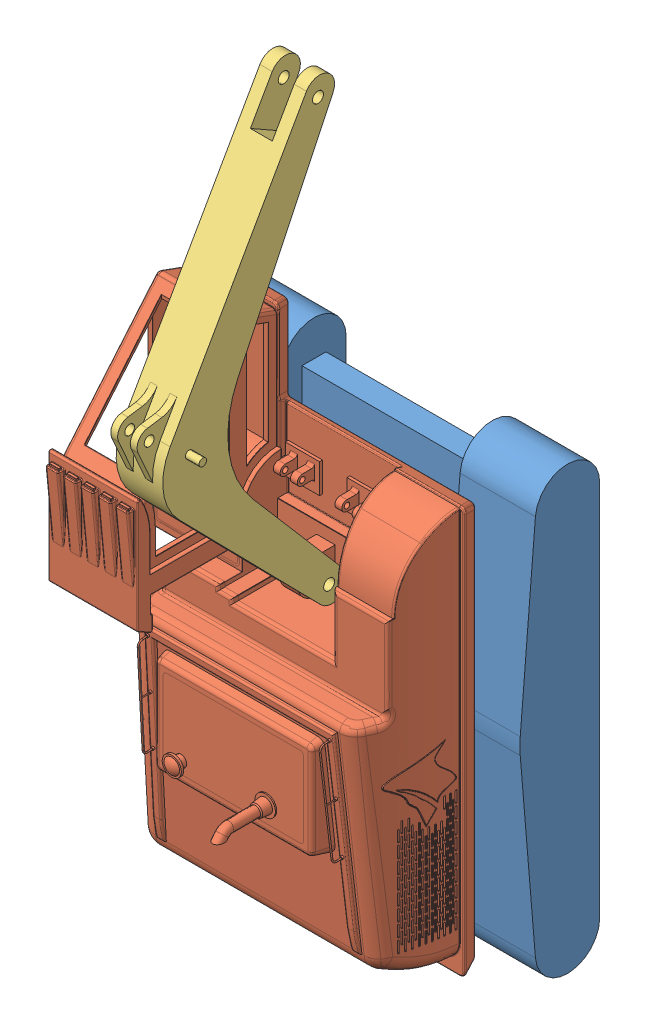
SolidWorks assembly MathScavator9000, configuration Default. Lengths in mm.
Overall size (4800 11116.11 4638.28).
3 component instances, 3 part files, 2 mates.
Components (placement in the parent):
- ExcavatorBase-1: ExcavatorBase [Default] at origin size (4800 6440 1295)
- Chassis_Primary_v2_PART-1: Chassis_Primary_v2_PART [Default] at origin size (3985.01 7287.04 2544.86)
- Boom-2: Boom [Default] at (3.9527 -17.4087 597.5917) x (0 0.999658 0.026161) z (1 0 0) size (6775.47 2834.12 1080)
Mates (geometry in assembly coordinates):
- Concentric1: concentric aligned: cylinder of Chassis_Primary_v2_PART-1 through (138.9527 -17.4087 597.5917) axis (1 0 0) radius 80; cylinder of Boom-2 through (343.9527 -17.4087 597.5917) axis (1 0 0) radius 80
- Distance1: distance = 25 mm anti-aligned: plane of Boom-2 through (-156.0473 -1732.805 1969.062) normal (1 0 0); plane of Chassis_Primary_v2_PART-1 through (-131.0473 -17.4087 597.5917) normal (-1 0 0)
